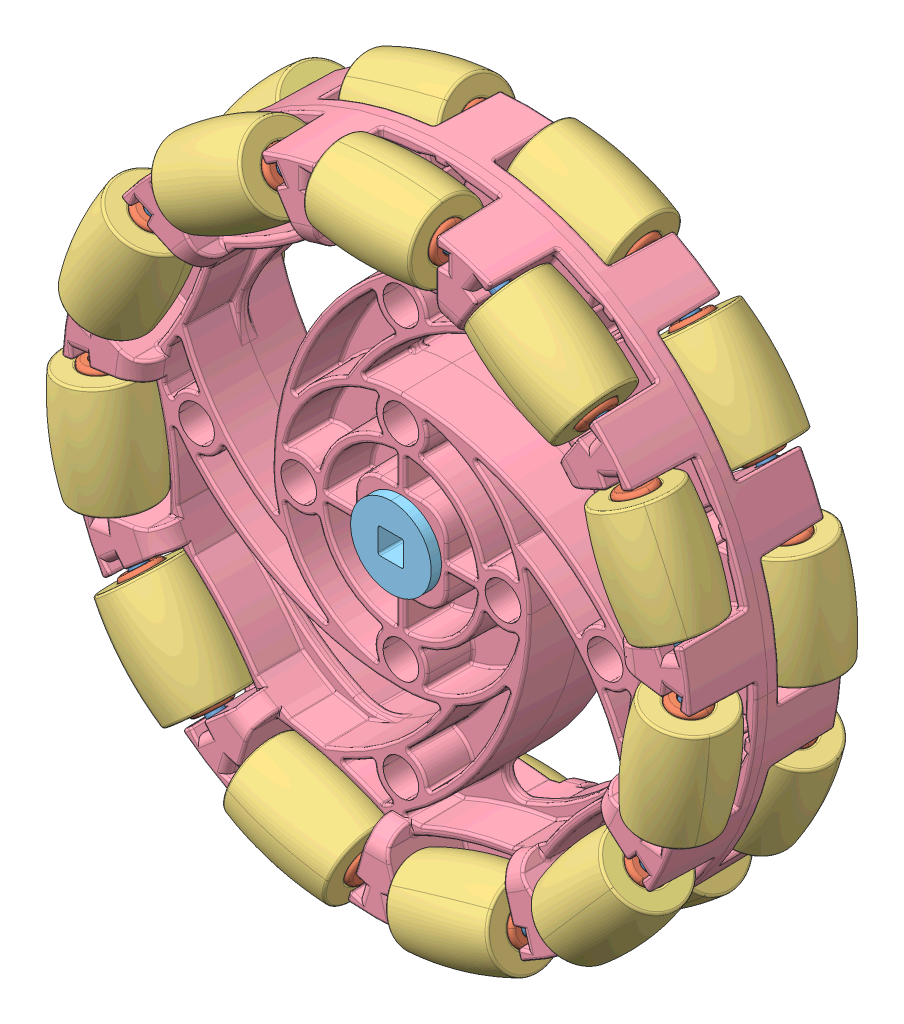
SolidWorks assembly 3.25in Omni With Inserts, configuration Default. Lengths in mm.
Overall size (90.82 89.11 34).
93 component instances, 5 part files, 6 mates.
Components (placement in the parent):
- 3.25_ Omni-Directional Wheel (276-3526) part-1: 3.25_ Omni-Directional Wheel (276-3526) part [Default] at (27.4232 51.2389 70.39) size (90.82 89.11 34)
  - 3.25_ Omni-Directional Wheel (276-3526) .step-1: 3.25_ Omni-Directional Wheel (276-3526) .step [Default] at origin size (90.82 89.11 34)
    - Roller Assembly.step-1: Roller Assembly.step [Default] at (-0.0014 35.9575 7.1) x (0 0.963098 -0.269151) z (-1 0 0) size (14.05 14.05 18.75)
      - 276-3526-001 Rev 1.step-1: 276-3526-001 Rev 1.step [Default] at origin size (2 2 18.75)
      - 276-3526-003 Rev 1.step-1: 276-3526-003 Rev 1.step [Default] at origin size (6.15 6.15 14.2)
      - 276-3526-002 Rev 1.step-1: 276-3526-002 Rev 1.step [Default] x (0 0 1) z (-0.908956 0.416893 0) size (13.2 10.6 10.6)
    - Roller Assembly.step-2: Roller Assembly.step [Default] at (-19.4287 30.2567 7.1) x (0.421057 -0.655178 0.627258) z (-0.841254 -0.540641 0) size (14.05 14.05 18.75)
      - 276-3526-001 Rev 1.step-1: 276-3526-001 Rev 1.step [Default] at origin size (2 2 18.75)
      - 276-3526-003 Rev 1.step-1: 276-3526-003 Rev 1.step [Default] at origin size (6.15 6.15 14.2)
      - 276-3526-002 Rev 1.step-1: 276-3526-002 Rev 1.step [Default] x (0 0 1) z (-0.908956 0.416893 0) size (13.2 10.6 10.6)
    - Roller Assembly.step-3: Roller Assembly.step [Default] at (-35.5935 -5.1038 7.1) x (0.979746 0.140866 -0.142315) z (0.142315 -0.989821 0) size (14.05 14.05 18.75)
      - 276-3526-001 Rev 1.step-1: 276-3526-001 Rev 1.step [Default] at origin size (2 2 18.75)
      - 276-3526-003 Rev 1.step-1: 276-3526-003 Rev 1.step [Default] at origin size (6.15 6.15 14.2)
      - 276-3526-002 Rev 1.step-1: 276-3526-002 Rev 1.step [Default] x (0 0 1) z (-0.908956 0.416893 0) size (13.2 10.6 10.6)
    - Roller Assembly.step-4: Roller Assembly.step [Default] at (-10.1434 -34.4972 7.1) x (0.079373 0.27032 -0.959493) z (0.959493 -0.281733 0) size (14.05 14.05 18.75)
      - 276-3526-001 Rev 1.step-1: 276-3526-001 Rev 1.step [Default] at origin size (2 2 18.75)
      - 276-3526-003 Rev 1.step-1: 276-3526-003 Rev 1.step [Default] at origin size (6.15 6.15 14.2)
      - 276-3526-002 Rev 1.step-1: 276-3526-002 Rev 1.step [Default] x (0 0 1) z (-0.908956 0.416893 0) size (13.2 10.6 10.6)
    - Roller Assembly.step-5: Roller Assembly.step [Default] at (27.166 -23.5574 7.1) x (-0.355209 0.30779 -0.882662) z (0.654861 0.75575 0) size (14.05 14.05 18.75)
      - 276-3526-001 Rev 1.step-1: 276-3526-001 Rev 1.step [Default] at origin size (2 2 18.75)
      - 276-3526-003 Rev 1.step-1: 276-3526-003 Rev 1.step [Default] at origin size (6.15 6.15 14.2)
      - 276-3526-002 Rev 1.step-1: 276-3526-002 Rev 1.step [Default] x (0 0 1) z (-0.908956 0.416893 0) size (13.2 10.6 10.6)
    - Roller Assembly.step-6: Roller Assembly.step [Default] at (32.7138 14.9249 7.1) x (0.89908 0.410596 0.151875) z (-0.415415 0.909632 0) size (14.05 14.05 18.75)
      - 276-3526-001 Rev 1.step-1: 276-3526-001 Rev 1.step [Default] at origin size (2 2 18.75)
      - 276-3526-003 Rev 1.step-1: 276-3526-003 Rev 1.step [Default] at origin size (6.15 6.15 14.2)
      - 276-3526-002 Rev 1.step-1: 276-3526-002 Rev 1.step [Default] x (0 0 1) z (-0.908956 0.416893 0) size (13.2 10.6 10.6)
    - Roller Assembly.step-7: Roller Assembly.step [Default] at (19.4515 30.242 7.1) x (0.194707 0.302971 0.932898) z (-0.841254 0.540641 0) size (14.05 14.05 18.75)
      - 276-3526-001 Rev 1.step-1: 276-3526-001 Rev 1.step [Default] at origin size (2 2 18.75)
      - 276-3526-003 Rev 1.step-1: 276-3526-003 Rev 1.step [Default] at origin size (6.15 6.15 14.2)
      - 276-3526-002 Rev 1.step-1: 276-3526-002 Rev 1.step [Default] x (0 0 1) z (-0.908956 0.416893 0) size (13.2 10.6 10.6)
    - Roller Assembly.step-8: Roller Assembly.step [Default] at (-32.7025 14.9497 7.1) x (0.82743 -0.377875 0.415415) z (-0.415415 -0.909632 0) size (14.05 14.05 18.75)
      - 276-3526-001 Rev 1.step-1: 276-3526-001 Rev 1.step [Default] at origin size (2 2 18.75)
      - 276-3526-003 Rev 1.step-1: 276-3526-003 Rev 1.step [Default] at origin size (6.15 6.15 14.2)
      - 276-3526-002 Rev 1.step-1: 276-3526-002 Rev 1.step [Default] x (0 0 1) z (-0.908956 0.416893 0) size (13.2 10.6 10.6)
    - Roller Assembly.step-9: Roller Assembly.step [Default] at (-27.1838 -23.5369 7.1) x (0.578931 0.501646 -0.642799) z (0.654861 -0.75575 0) size (14.05 14.05 18.75)
      - 276-3526-001 Rev 1.step-1: 276-3526-001 Rev 1.step [Default] at origin size (2 2 18.75)
      - 276-3526-003 Rev 1.step-1: 276-3526-003 Rev 1.step [Default] at origin size (6.15 6.15 14.2)
      - 276-3526-002 Rev 1.step-1: 276-3526-002 Rev 1.step [Default] x (0 0 1) z (-0.908956 0.416893 0) size (13.2 10.6 10.6)
    - Roller Assembly.step-10: Roller Assembly.step [Default] at (10.1174 -34.5048 7.1) x (0.079373 -0.27032 -0.959493) z (0.959493 0.281733 0) size (14.05 14.05 18.75)
      - 276-3526-001 Rev 1.step-1: 276-3526-001 Rev 1.step [Default] at origin size (2 2 18.75)
      - 276-3526-003 Rev 1.step-1: 276-3526-003 Rev 1.step [Default] at origin size (6.15 6.15 14.2)
      - 276-3526-002 Rev 1.step-1: 276-3526-002 Rev 1.step [Default] x (0 0 1) z (-0.908956 0.416893 0) size (13.2 10.6 10.6)
    - Roller Assembly.step-11: Roller Assembly.step [Default] at (35.5896 -5.1307 7.1) x (0.988515 -0.142127 -0.05136) z (0.142315 0.989821 0) size (14.05 14.05 18.75)
      - 276-3526-001 Rev 1.step-1: 276-3526-001 Rev 1.step [Default] at origin size (2 2 18.75)
      - 276-3526-003 Rev 1.step-1: 276-3526-003 Rev 1.step [Default] at origin size (6.15 6.15 14.2)
      - 276-3526-002 Rev 1.step-1: 276-3526-002 Rev 1.step [Default] x (0 0 1) z (-0.908956 0.416893 0) size (13.2 10.6 10.6)
    - Roller Assembly.step-12: Roller Assembly.step [Default] at (10.1434 34.4972 -7.1) x (0.083119 0.283078 -0.955489) z (0.959493 -0.281733 0) size (14.05 14.05 18.75)
      - 276-3526-001 Rev 1.step-1: 276-3526-001 Rev 1.step [Default] at origin size (2 2 18.75)
      - 276-3526-003 Rev 1.step-1: 276-3526-003 Rev 1.step [Default] at origin size (6.15 6.15 14.2)
      - 276-3526-002 Rev 1.step-1: 276-3526-002 Rev 1.step [Default] x (0 0 1) z (-0.908956 0.416893 0) size (13.2 10.6 10.6)
    - Roller Assembly.step-13: Roller Assembly.step [Default] at (27.1838 23.5369 -7.1) x (0.582526 0.504762 -0.637086) z (0.654861 -0.75575 0) size (14.05 14.05 18.75)
      - 276-3526-001 Rev 1.step-1: 276-3526-001 Rev 1.step [Default] at origin size (2 2 18.75)
      - 276-3526-003 Rev 1.step-1: 276-3526-003 Rev 1.step [Default] at origin size (6.15 6.15 14.2)
      - 276-3526-002 Rev 1.step-1: 276-3526-002 Rev 1.step [Default] x (0 0 1) z (-0.908956 0.416893 0) size (13.2 10.6 10.6)
    - Roller Assembly.step-14: Roller Assembly.step [Default] at (35.5935 5.1038 -7.1) x (0.926341 0.133188 -0.352355) z (0.142315 -0.989821 0) size (14.05 14.05 18.75)
      - 276-3526-001 Rev 1.step-1: 276-3526-001 Rev 1.step [Default] at origin size (2 2 18.75)
      - 276-3526-003 Rev 1.step-1: 276-3526-003 Rev 1.step [Default] at origin size (6.15 6.15 14.2)
      - 276-3526-002 Rev 1.step-1: 276-3526-002 Rev 1.step [Default] x (0 0 1) z (-0.908956 0.416893 0) size (13.2 10.6 10.6)
    - Roller Assembly.step-15: Roller Assembly.step [Default] at (32.7025 -14.9497 -7.1) x (0.897398 -0.409828 0.163453) z (-0.415415 -0.909632 0) size (14.05 14.05 18.75)
      - 276-3526-001 Rev 1.step-1: 276-3526-001 Rev 1.step [Default] at origin size (2 2 18.75)
      - 276-3526-003 Rev 1.step-1: 276-3526-003 Rev 1.step [Default] at origin size (6.15 6.15 14.2)
      - 276-3526-002 Rev 1.step-1: 276-3526-002 Rev 1.step [Default] x (0 0 1) z (-0.908956 0.416893 0) size (13.2 10.6 10.6)
    - Roller Assembly.step-16: Roller Assembly.step [Default] at (19.4287 -30.2567 -7.1) x (0.277612 -0.431972 0.858098) z (-0.841254 -0.540641 0) size (14.05 14.05 18.75)
      - 276-3526-001 Rev 1.step-1: 276-3526-001 Rev 1.step [Default] at origin size (2 2 18.75)
      - 276-3526-003 Rev 1.step-1: 276-3526-003 Rev 1.step [Default] at origin size (6.15 6.15 14.2)
      - 276-3526-002 Rev 1.step-1: 276-3526-002 Rev 1.step [Default] x (0 0 1) z (-0.908956 0.416893 0) size (13.2 10.6 10.6)
    - Roller Assembly.step-17: Roller Assembly.step [Default] at (-0.0136 -35.9575 -7.1) x (0 -0.239919 0.970793) z (-1 0 0) size (14.05 14.05 18.75)
      - 276-3526-001 Rev 1.step-1: 276-3526-001 Rev 1.step [Default] at origin size (2 2 18.75)
      - 276-3526-003 Rev 1.step-1: 276-3526-003 Rev 1.step [Default] at origin size (6.15 6.15 14.2)
      - 276-3526-002 Rev 1.step-1: 276-3526-002 Rev 1.step [Default] x (0 0 1) z (-0.908956 0.416893 0) size (13.2 10.6 10.6)
    - Roller Assembly.step-18: Roller Assembly.step [Default] at (-19.4515 -30.242 -7.1) x (0.31008 0.482494 0.819176) z (-0.841254 0.540641 0) size (14.05 14.05 18.75)
      - 276-3526-001 Rev 1.step-1: 276-3526-001 Rev 1.step [Default] at origin size (2 2 18.75)
      - 276-3526-003 Rev 1.step-1: 276-3526-003 Rev 1.step [Default] at origin size (6.15 6.15 14.2)
      - 276-3526-002 Rev 1.step-1: 276-3526-002 Rev 1.step [Default] x (0 0 1) z (-0.908956 0.416893 0) size (13.2 10.6 10.6)
    - Roller Assembly.step-19: Roller Assembly.step [Default] at (-32.7138 -14.9249 -7.1) x (0.58758 0.268339 0.763377) z (-0.415415 0.909632 0) size (14.05 14.05 18.75)
      - 276-3526-001 Rev 1.step-1: 276-3526-001 Rev 1.step [Default] at origin size (2 2 18.75)
      - 276-3526-003 Rev 1.step-1: 276-3526-003 Rev 1.step [Default] at origin size (6.15 6.15 14.2)
      - 276-3526-002 Rev 1.step-1: 276-3526-002 Rev 1.step [Default] x (0 0 1) z (-0.908956 0.416893 0) size (13.2 10.6 10.6)
    - Roller Assembly.step-20: Roller Assembly.step [Default] at (-35.5896 5.1307 -7.1) x (0.965498 -0.138818 0.220323) z (0.142315 0.989821 0) size (14.05 14.05 18.75)
      - 276-3526-001 Rev 1.step-1: 276-3526-001 Rev 1.step [Default] at origin size (2 2 18.75)
      - 276-3526-003 Rev 1.step-1: 276-3526-003 Rev 1.step [Default] at origin size (6.15 6.15 14.2)
      - 276-3526-002 Rev 1.step-1: 276-3526-002 Rev 1.step [Default] x (0 0 1) z (-0.908956 0.416893 0) size (13.2 10.6 10.6)
    - Roller Assembly.step-21: Roller Assembly.step [Default] at (-27.166 23.5574 -7.1) x (0.75327 -0.652712 -0.080935) z (0.654861 0.75575 0) size (14.05 14.05 18.75)
      - 276-3526-001 Rev 1.step-1: 276-3526-001 Rev 1.step [Default] at origin size (2 2 18.75)
      - 276-3526-003 Rev 1.step-1: 276-3526-003 Rev 1.step [Default] at origin size (6.15 6.15 14.2)
      - 276-3526-002 Rev 1.step-1: 276-3526-002 Rev 1.step [Default] x (0 0 1) z (-0.908956 0.416893 0) size (13.2 10.6 10.6)
    - Roller Assembly.step-22: Roller Assembly.step [Default] at (-10.1174 34.5048 -7.1) x (0.123782 -0.421563 -0.898311) z (0.959493 0.281733 0) size (14.05 14.05 18.75)
      - 276-3526-001 Rev 1.step-1: 276-3526-001 Rev 1.step [Default] at origin size (2 2 18.75)
      - 276-3526-003 Rev 1.step-1: 276-3526-003 Rev 1.step [Default] at origin size (6.15 6.15 14.2)
      - 276-3526-002 Rev 1.step-1: 276-3526-002 Rev 1.step [Default] x (0 0 1) z (-0.908956 0.416893 0) size (13.2 10.6 10.6)
    - 276-3526-004 Rev 1.step-1: 276-3526-004 Rev 1.step [Default] at origin size (78.5 78.5 19.07)
- Metal Shaft Inserts (276-3881-002)-1: Metal Shaft Inserts (276-3881-002) [Default] at (27.4486 51.2643 62.77) x (0 1 0) z (1 0 0) size (10.03 5.08 10.03)
- Metal Shaft Inserts (276-3881-002)-2: Metal Shaft Inserts (276-3881-002) [Default] at (27.4486 51.2643 78.01) x (1 0 0) z (0 1 0) size (10.03 5.08 10.03)
Mates (geometry in assembly coordinates):
- Coincident1: coincident anti-aligned: plane of 3.25_ Omni-Directional Wheel (276-3526) part-1/3.25_ Omni-Directional Wheel (276-3526) .step-1/276-3526-004 Rev 1.step-1 through (24.2482 54.4139 60.865) normal (0 -1 0); plane of Metal Shaft Inserts (276-3881-002)-2 through (24.299 54.4139 72.93) normal (0 1 0)
- Coincident2: coincident anti-aligned: plane of 3.25_ Omni-Directional Wheel (276-3526) part-1/3.25_ Omni-Directional Wheel (276-3526) .step-1/276-3526-004 Rev 1.step-1 through (30.5982 54.4139 60.865) normal (-1 0 0); plane of Metal Shaft Inserts (276-3881-002)-2 through (30.5982 48.1147 72.93) normal (1 0 0)
- Coincident3: coincident anti-aligned: plane of 3.25_ Omni-Directional Wheel (276-3526) part-1/3.25_ Omni-Directional Wheel (276-3526) .step-1/276-3526-004 Rev 1.step-1 through (27.4232 51.2389 76.74) normal (0 0 1); plane of Metal Shaft Inserts (276-3881-002)-2 through (27.4486 51.2643 76.74) normal (0 0 -1)
- Coincident4: coincident anti-aligned: plane of 3.25_ Omni-Directional Wheel (276-3526) part-1/3.25_ Omni-Directional Wheel (276-3526) .step-1/276-3526-004 Rev 1.step-1 through (30.5982 54.4139 60.865) normal (-1 0 0); plane of Metal Shaft Inserts (276-3881-002)-1 through (30.5982 48.1147 67.85) normal (1 0 0)
- Coincident5: coincident anti-aligned: plane of 3.25_ Omni-Directional Wheel (276-3526) part-1/3.25_ Omni-Directional Wheel (276-3526) .step-1/276-3526-004 Rev 1.step-1 through (24.2482 54.4139 60.865) normal (0 -1 0); plane of Metal Shaft Inserts (276-3881-002)-1 through (24.299 54.4139 67.85) normal (0 1 0)
- Coincident6: coincident anti-aligned: plane of 3.25_ Omni-Directional Wheel (276-3526) part-1/3.25_ Omni-Directional Wheel (276-3526) .step-1/276-3526-004 Rev 1.step-1 through (27.4232 51.2389 64.04) normal (0 0 -1); plane of Metal Shaft Inserts (276-3881-002)-1 through (27.4486 51.2643 64.04) normal (0 0 1)
